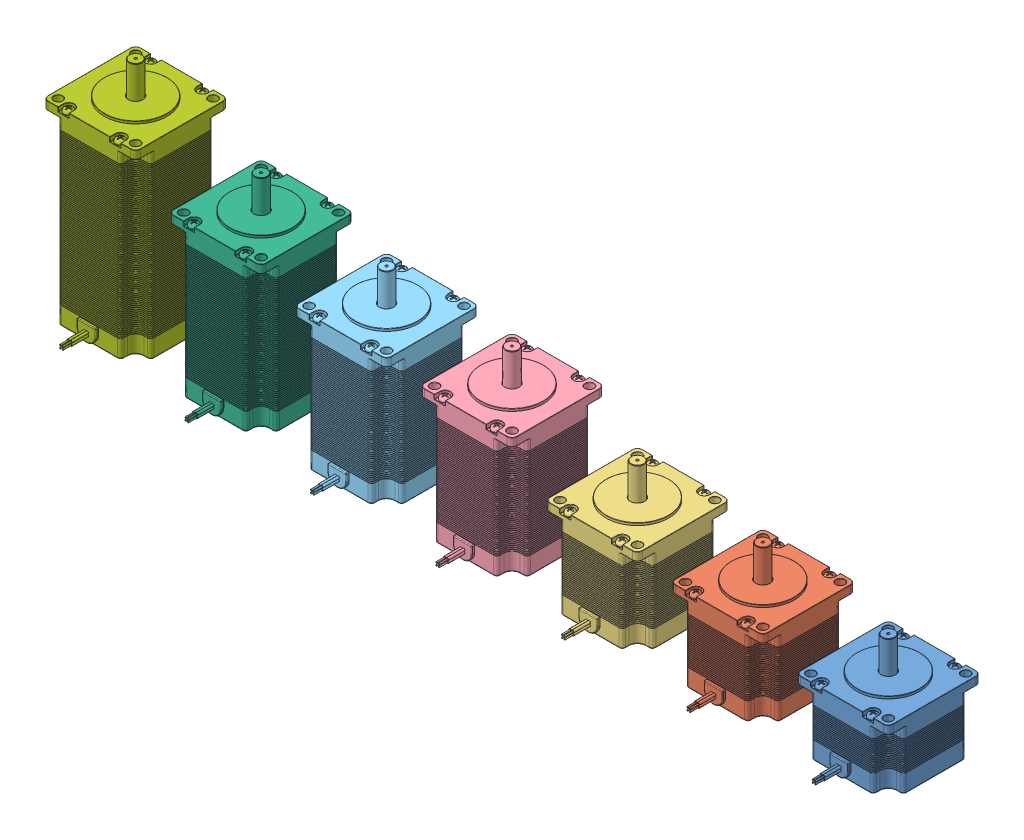
SolidWorks assembly Nema 23 Stepper Motor length 41-115mm, configuration По умолчанию. Lengths in mm.
Overall size (514.26 135.5 73.38).
7 component instances, 7 part files, 20 mates.
Components (placement in the parent):
- Nema 23 Stepper Motor length 41mm-1: Nema 23 Stepper Motor length 41mm [По умолчанию] at origin size (56.46 61.5 73.38)
- Nema 23 Stepper Motor length 51mm-1: Nema 23 Stepper Motor length 51mm [По умолчанию] at (-76.3 0 0) size (56.46 71.5 73.38)
- Nema 23 Stepper Motor length 56mm-1: Nema 23 Stepper Motor length 56mm [По умолчанию] at (-152.6 0 0) size (56.46 76.5 73.38)
- Nema 23 Stepper Motor length 78mm-1: Nema 23 Stepper Motor length 78mm [По умолчанию] at (-228.9 0 0) size (56.46 98.5 73.38)
- Nema 23 Stepper Motor length 82mm-1: Nema 23 Stepper Motor length 82mm [По умолчанию] at (-305.2 0 0) size (56.46 102.5 73.38)
- Nema 23 Stepper Motor length 93mm-1: Nema 23 Stepper Motor length 93mm [По умолчанию] at (-381.5 0 0) size (56.46 113.5 73.38)
- Nema 23 Stepper Motor length 115mm-1: Nema 23 Stepper Motor length 115mm [По умолчанию] at (-457.8 0 0) size (56.46 135.5 73.38)
Mates (geometry in assembly coordinates):
- Совпадение1: coincident aligned: plane of Nema 23 Stepper Motor length 41mm-1 through (0 11 28.15) normal (0 0 1); plane of Nema 23 Stepper Motor length 51mm-1 through (-76.3 11 28.15) normal (0 0 1)
- Совпадение2: coincident aligned: plane of Nema 23 Stepper Motor length 51mm-1 through (-76.3 11 28.15) normal (0 0 1); plane of Nema 23 Stepper Motor length 56mm-1 through (-152.6 11 28.15) normal (0 0 1)
- Совпадение3: coincident aligned: plane of Nema 23 Stepper Motor length 56mm-1 through (-152.6 11 28.15) normal (0 0 1); plane of Nema 23 Stepper Motor length 78mm-1 through (-228.9 11 28.15) normal (0 0 1)
- Совпадение4: coincident aligned: plane of Nema 23 Stepper Motor length 93mm-1 through (-381.5 11 28.15) normal (0 0 1); plane of Nema 23 Stepper Motor length 115mm-1 through (-457.8 11 28.15) normal (0 0 1)
- Совпадение5: coincident aligned: plane of Nema 23 Stepper Motor length 82mm-1 through (-305.2 11 28.15) normal (0 0 1); plane of Nema 23 Stepper Motor length 93mm-1 through (-381.5 11 28.15) normal (0 0 1)
- Совпадение6: coincident aligned: plane of Nema 23 Stepper Motor length 78mm-1 through (-228.9 11 28.15) normal (0 0 1); plane of Nema 23 Stepper Motor length 82mm-1 through (-305.2 11 28.15) normal (0 0 1)
- Совпадение7: coincident aligned: plane of Nema 23 Stepper Motor length 56mm-1 through (-152.6 11 28.15) normal (0 0 1); plane of Nema 23 Stepper Motor length 78mm-1 through (-228.9 11 28.15) normal (0 0 1)
- Совпадение8: coincident aligned: plane of Nema 23 Stepper Motor length 51mm-1 through (-76.3 11 28.15) normal (0 0 1); plane of Nema 23 Stepper Motor length 56mm-1 through (-152.6 11 28.15) normal (0 0 1)
- Совпадение9: coincident aligned: plane of Nema 23 Stepper Motor length 41mm-1 through (0 0 0) normal (0 -1 0); plane of Nema 23 Stepper Motor length 51mm-1 through (-76.3 0 0) normal (0 -1 0)
- Совпадение10: coincident aligned: plane of Nema 23 Stepper Motor length 51mm-1 through (-76.3 0 0) normal (0 -1 0); plane of Nema 23 Stepper Motor length 56mm-1 through (-152.6 0 0) normal (0 -1 0)
- Совпадение11: coincident aligned: plane of Nema 23 Stepper Motor length 56mm-1 through (-152.6 0 0) normal (0 -1 0); plane of Nema 23 Stepper Motor length 78mm-1 through (-228.9 0 0) normal (0 -1 0)
- Совпадение12: coincident aligned: plane of Nema 23 Stepper Motor length 78mm-1 through (-228.9 0 0) normal (0 -1 0); plane of Nema 23 Stepper Motor length 82mm-1 through (-305.2 0 0) normal (0 -1 0)
- Совпадение13: coincident aligned: plane of Nema 23 Stepper Motor length 82mm-1 through (-305.2 0 0) normal (0 -1 0); plane of Nema 23 Stepper Motor length 93mm-1 through (-381.5 0 0) normal (0 -1 0)
- Совпадение14: coincident aligned: plane of Nema 23 Stepper Motor length 93mm-1 through (-381.5 0 0) normal (0 -1 0); plane of Nema 23 Stepper Motor length 115mm-1 through (-457.8 0 0) normal (0 -1 0)
- Расстояние1: distance = 20 mm anti-aligned: plane of Nema 23 Stepper Motor length 41mm-1 through (-28.15 11 0) normal (-1 0 0); plane of Nema 23 Stepper Motor length 51mm-1 through (-48.15 11 0) normal (1 0 0)
- Расстояние2: distance = 20 mm anti-aligned: plane of Nema 23 Stepper Motor length 56mm-1 through (-124.45 11 0) normal (1 0 0); plane of Nema 23 Stepper Motor length 51mm-1 through (-104.45 11 0) normal (-1 0 0)
- Расстояние3: distance = 20 mm anti-aligned: plane of Nema 23 Stepper Motor length 56mm-1 through (-180.75 11 0) normal (-1 0 0); plane of Nema 23 Stepper Motor length 78mm-1 through (-200.75 11 0) normal (1 0 0)
- Расстояние4: distance = 20 mm anti-aligned: plane of Nema 23 Stepper Motor length 82mm-1 through (-277.05 11 0) normal (1 0 0); plane of Nema 23 Stepper Motor length 78mm-1 through (-257.05 11 0) normal (-1 0 0)
- Расстояние5: distance = 20 mm anti-aligned: plane of Nema 23 Stepper Motor length 82mm-1 through (-333.35 11 0) normal (-1 0 0); plane of Nema 23 Stepper Motor length 93mm-1 through (-353.35 11 0) normal (1 0 0)
- Расстояние6: distance = 20 mm anti-aligned: plane of Nema 23 Stepper Motor length 115mm-1 through (-429.65 11 0) normal (1 0 0); plane of Nema 23 Stepper Motor length 93mm-1 through (-409.65 11 0) normal (-1 0 0)
